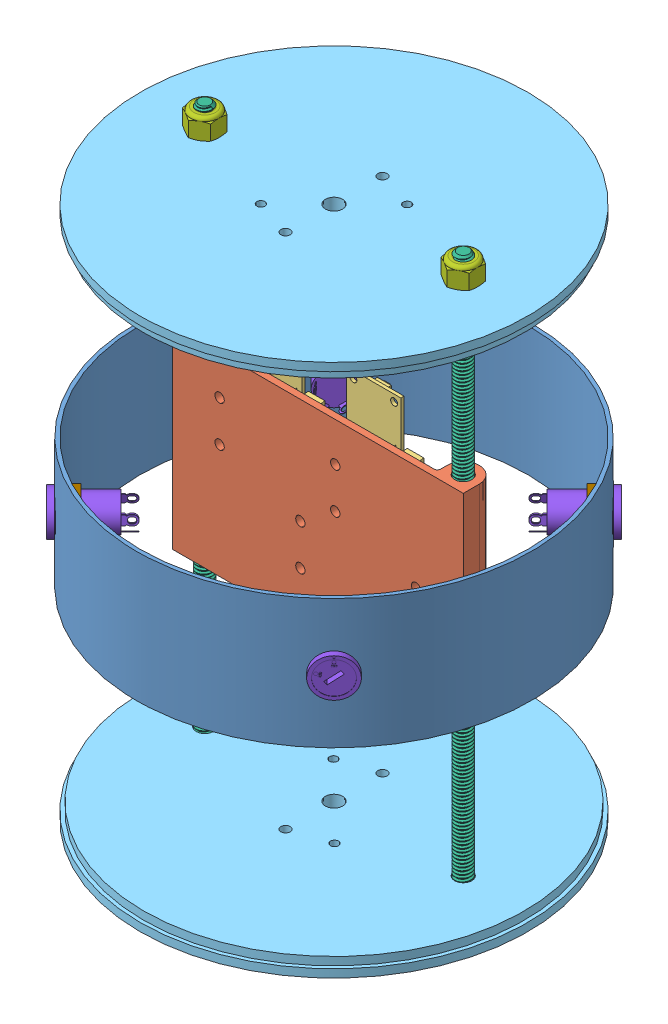
SolidWorks assembly Recovery Bay, configuration Default. Lengths in mm.
Overall size (155.24 228.76 155.24).
24 component instances, 10 part files, 22 mates.
Components (placement in the parent):
- Recovery Band-1: Recovery Band [Default] at origin size (155.24 50.8 155.24)
- Recovery Coupler-1: Recovery Coupler [Default] at origin size (152.4 203.2 152.4) (hidden)
- Recovery_sled_assm-1: Recovery_sled_assm [Default] at origin size (114.3 108.1 19.04)
  - Recovery Sled(new)-1: Recovery Sled(new) [Default] at origin size (114.3 76.53 12.7)
  - altimeter-1: altimeter [Default] at (19.431 30.353 3.81) x (1 0 0) z (0 1 0) size (21.34 10.79 50.8)
  - bat_9v.step-1: bat_9v.step [Default] at (19.431 -52.345 -4.44) x (1 0 0) z (0 1 0) size (25.3 16.5 47.8)
  - bat_9v.step-2: bat_9v.step [Default] at (-19.431 -52.345 -4.44) x (-1 0 0) z (0 1 0) size (25.3 16.5 47.8)
  - altimeter-2: altimeter [Default] at (-19.431 30.353 3.81) x (1 0 0) z (0 1 0) size (21.34 10.79 50.8)
- cap-1: cap [Default] at (0 103.1875 0) x (-1 0 0) z (0 0 1) size (152.4 6.35 152.4)
- 3313N11_High-Strength Steel Threaded Rod-1: 3313N11_High-Strength Steel Threaded Rod [3313N11] at (50.8 0 -3.175) x (1 0 0) z (0 1 0) size (6.42 7.35 228.76)
- 90630A110_High-Strength Steel Nylon-Insert Locknut-1: 90630A110_High-Strength Steel Nylon-Insert Locknut [90630A110] at (50.8 104.775 0) size (11.11 8.31 12.83)
- 90630A110_High-Strength Steel Nylon-Insert Locknut-2: 90630A110_High-Strength Steel Nylon-Insert Locknut [90630A110] at (-50.8 104.775 0) x (-1 0 0) z (0 0 -1) size (11.11 8.31 12.83)
- 3313N11_High-Strength Steel Threaded Rod-2: 3313N11_High-Strength Steel Threaded Rod [3313N11] at (-50.8 0 3.175) x (-1 0 0) z (0 1 0) size (6.42 7.35 228.76)
- 90630A110_High-Strength Steel Nylon-Insert Locknut-3: 90630A110_High-Strength Steel Nylon-Insert Locknut [90630A110] at (-50.8 -104.775 0) x (-1 0 0) z (0 0 1) size (11.11 8.31 12.83)
- 90630A110_High-Strength Steel Nylon-Insert Locknut-4: 90630A110_High-Strength Steel Nylon-Insert Locknut [90630A110] at (50.8 -104.775 0) x (1 0 0) z (0 0 -1) size (11.11 8.31 12.83)
- cap-2: cap [Default] at (0 -103.1875 0) x (-1 0 0) z (0 0 -1) size (152.4 6.35 152.4)
- rotary_swtich-1: rotary_swtich [Default] at (-55.7005 0 55.7005) x (0.707107 0 0.707107) z (0 -1 0) size (15.2 25.8 15.2)
- rotary_swtich_nut-1: rotary_swtich_nut [Default] at (-52.6522 0 52.6522) x (-0.707107 0 -0.707107) z (0 -1 0) size (15.88 4.57 15.88)
- rotary_swtich-2: rotary_swtich [Default] at (-55.7005 0 -55.7005) x (-0.707107 0 0.707107) z (0 -1 0) size (15.2 25.8 15.2)
- rotary_swtich-3: rotary_swtich [Default] at (55.7005 0 -55.7005) x (-0.707107 0 -0.707107) z (0 -1 0) size (15.2 25.8 15.2)
- rotary_swtich-4: rotary_swtich [Default] at (55.7005 0 55.7005) x (0.707107 0 -0.707107) z (0 -1 0) size (15.2 25.8 15.2)
- rotary_swtich_nut-2: rotary_swtich_nut [Default] at (-52.6522 0 -52.6522) x (0.707107 0 -0.707107) z (0 -1 0) size (15.88 4.57 15.88)
- rotary_swtich_nut-3: rotary_swtich_nut [Default] at (52.6522 0 -52.6522) x (0.707107 0 0.707107) z (0 -1 0) size (15.88 4.57 15.88)
- rotary_swtich_nut-4: rotary_swtich_nut [Default] at (52.6522 0 52.6522) x (-0.707107 0 0.707107) z (0 -1 0) size (15.88 4.57 15.88)
Mates (geometry in assembly coordinates):
- Coincident1: coincident aligned: plane of Recovery Band-1 through (0 0 0) normal (0 0 1)
- Coincident2: coincident aligned: plane of Recovery Band-1 through (0 0 0) normal (0 1 0)
- Coincident3: coincident aligned: plane of Recovery Band-1 through (0 0 0) normal (1 0 0)
- Coincident4: coincident aligned: plane of Recovery Band-1 through (0 0 0) normal (0 0 1); plane of Recovery Coupler-1 through (0 0 0) normal (0 0 1)
- Coincident5: coincident aligned: plane of Recovery Band-1 through (0 0 0) normal (0 1 0); plane of Recovery Coupler-1 through (0 0 0) normal (0 1 0)
- Coincident6: coincident aligned: plane of Recovery Band-1 through (0 0 0) normal (1 0 0); plane of Recovery Coupler-1 through (0 0 0) normal (1 0 0)
- Coincident7: coincident aligned: plane of Recovery_sled_assm-1 through (0 0 0) normal (0 0 1)
- Coincident8: coincident aligned: plane of Recovery_sled_assm-1 through (0 0 0) normal (0 1 0)
- Coincident9: coincident aligned: plane of Recovery_sled_assm-1 through (0 0 0) normal (1 0 0)
- Coincident10: coincident anti-aligned: plane of Recovery Coupler-1 through (0 101.6 0) normal (0 1 0); plane of cap-1 through (0 101.6 0) normal (0 -1 0)
- Concentric1: concentric anti-aligned: circle of Recovery Coupler-1; circle of cap-1
- Coincident12: coincident aligned: plane of cap-1 through (0 103.1875 0) normal (0 0 1)
- Concentric2: concentric anti-aligned: circle of Recovery_sled_assm-1/Recovery Sled(new)-1; circle of 3313N11_High-Strength Steel Threaded Rod-1
- Coincident13: coincident aligned: plane of 3313N11_High-Strength Steel Threaded Rod-1 through (50.8 0 -3.175) normal (0 1 0)
- Concentric3: concentric anti-aligned: circle of 3313N11_High-Strength Steel Threaded Rod-1; circle of 90630A110_High-Strength Steel Nylon-Insert Locknut-1
- Coincident14: coincident anti-aligned: plane of cap-1 through (0 104.775 0) normal (0 1 0); plane of 90630A110_High-Strength Steel Nylon-Insert Locknut-1 through (56.3562 104.775 -3.2079) normal (0 -1 0)
- Tangent1: tangent anti-aligned: cylinder of Recovery Band-1 through (0 25.4 0) axis (0 -1 0) radius 77.6224; plane of rotary_swtich-1 through (-54.8873 0 54.8873) normal (0.707107 0 -0.707107)
- Coincident15: coincident aligned: axis of Recovery Band-1 through (-53.6941 0 53.6941) axis (-0.707107 0 0.707107); line of rotary_swtich-1 through (-41.8058 0 41.8058) axis (-0.707107 0 0.707107)
- Coincident16: coincident anti-aligned: plane of Recovery_sled_assm-1 through (0 0 0) normal (0 1 0); plane of rotary_swtich-1 through (-55.7005 0 55.7005) normal (0 -1 0)
- Coincident17: coincident anti-aligned: line of rotary_swtich-1 through (-41.8058 0 41.8058) axis (-0.707107 0 0.707107); line of rotary_swtich_nut-1 through (-52.9216 0 52.9216) axis (0.707107 0 -0.707107)
- Distance1: distance = 5.08 mm aligned: plane of rotary_swtich_nut-1 through (-52.9216 0 52.9216) normal (-0.707107 0 0.707107); plane of rotary_swtich-1 through (-56.5137 0 56.5137) normal (-0.707107 0 0.707107)
- Coincident19: coincident anti-aligned: plane of rotary_swtich-1 through (-55.7005 0 55.7005) normal (0.707107 0 0.707107); plane of rotary_swtich_nut-1 through (-52.6522 0 52.6522) normal (-0.707107 0 -0.707107)
